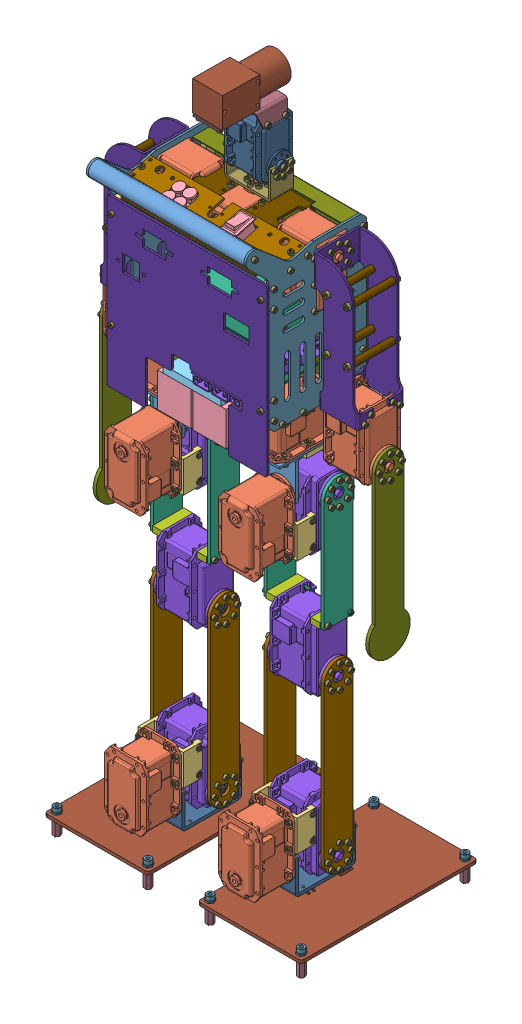
SolidWorks assembly 机器人, configuration 默认. Lengths in mm. (continued)
Components (placement in the parent): (continued)
- 左腿-1: 左腿 [默认] at (1223.8429 -132.4302 49.3314) x (0.483512 -0.009844 -0.875282) z (0.842178 0.277849 0.4621) size (197.18 402.23 253.32) (continued)
  - hexagon socket head cap screws gb-41: hexagon socket head cap screws gb [GB_FASTENER_SCREWS_HSHCS M2.5X6-N] at (-141.6338 221.8483 -139.9557) x (-0.009844 0.960574 0.277849) z (-0.277849 -0.269548 0.922033) size (8.5 4.5 4.5)
  - hexagon socket head cap screws gb-42: hexagon socket head cap screws gb [GB_FASTENER_SCREWS_HSHCS M2.5X6-N] at (-152.2711 227.0985 -158.4836) x (-0.009844 0.960574 0.277849) z (-0.277849 -0.269548 0.922033) size (8.5 4.5 4.5)
  - hexagon socket head cap screws gb-43: hexagon socket head cap screws gb [GB_FASTENER_SCREWS_HSHCS M2.5X6-N] at (-124.262 231.6628 -173.2708) x (-0.009844 0.960574 0.277849) z (-0.277849 -0.269548 0.922033) size (8.5 4.5 4.5)
  - hexagon socket head cap screws gb-44: hexagon socket head cap screws gb [GB_FASTENER_SCREWS_HSHCS M2.5X6-N] at (-113.6248 226.4125 -154.7429) x (-0.009844 0.960574 0.277849) z (-0.277849 -0.269548 0.922033) size (8.5 4.5 4.5)
  - hexagon socket head cap screws gb-45: hexagon socket head cap screws gb [GB_FASTENER_SCREWS_HSHCS M2.5X6-N] at (-151.57 247.2943 -140.1019) x (-0.875282 -0.142634 0.4621) z (-0.4621 0.528483 -0.712158) size (8.5 4.5 4.5)
  - hexagon socket head cap screws gb-46: hexagon socket head cap screws gb [GB_FASTENER_SCREWS_HSHCS M2.5X6-N] at (-147.8409 248.5328 -132.6561) x (-0.875282 -0.142634 0.4621) z (-0.4621 0.528483 -0.712158) size (8.5 4.5 4.5)
  - hexagon socket head cap screws gb-47: hexagon socket head cap screws gb [GB_FASTENER_SCREWS_HSHCS M2.5X6-N] at (-146.3597 255.2355 -127.7816) x (-0.875282 -0.142634 0.4621) z (-0.4621 0.528483 -0.712158) size (8.5 4.5 4.5)
  - hexagon socket head cap screws gb-50: hexagon socket head cap screws gb [GB_FASTENER_SCREWS_HSHCS M2.5X6-N] at (-150.9798 554.3402 -44.2096) x (-0.875282 -0.142634 0.4621) z (-0.4621 0.528483 -0.712158) size (8.5 4.5 4.5)
  - hexagon socket head cap screws gb-51: hexagon socket head cap screws gb [GB_FASTENER_SCREWS_HSHCS M2.5X6-N] at (-154.7723 559.2912 -49.865) x (-0.875282 -0.142634 0.4621) z (-0.4621 0.528483 -0.712158) size (8.5 4.5 4.5)
  - hexagon socket head cap screws gb-52: hexagon socket head cap screws gb [GB_FASTENER_SCREWS_HSHCS M2.5X6-N] at (-149.3454 546.0998 -43.6574) x (-0.875282 -0.142634 0.4621) z (-0.4621 0.528483 -0.712158) size (8.5 4.5 4.5)
  - hexagon socket head cap screws gb-54: hexagon socket head cap screws gb [GB_FASTENER_SCREWS_HSHCS M2.5X6-N] at (-141.4858 262.0369 -179.1169) x (0.483512 -0.238647 0.842178) z (-0.842178 0.135478 0.521902) size (8.5 4.5 4.5)
  - hexagon socket head cap screws gb-55: hexagon socket head cap screws gb [GB_FASTENER_SCREWS_HSHCS M2.5X6-N] at (-138.7424 269.9679 -178.4445) x (0.483512 -0.238647 0.842178) z (-0.842178 0.135478 0.521902) size (8.5 4.5 4.5)
  - hexagon socket head cap screws gb-56: hexagon socket head cap screws gb [GB_FASTENER_SCREWS_HSHCS M2.5X6-N] at (-141.6389 276.9799 -174.7946) x (0.483512 -0.238647 0.842178) z (-0.842178 0.135478 0.521902) size (8.5 4.5 4.5)
  - hexagon socket head cap screws gb-57: hexagon socket head cap screws gb [GB_FASTENER_SCREWS_HSHCS M2.5X6-N] at (-148.4787 278.9653 -170.3051) x (0.483512 -0.238647 0.842178) z (-0.842178 0.135478 0.521902) size (8.5 4.5 4.5)
  - hexagon socket head cap screws gb-58: hexagon socket head cap screws gb [GB_FASTENER_SCREWS_HSHCS M2.5X6-N] at (-148.2622 257.8326 -176.4177) x (0.483512 -0.238647 0.842178) z (-0.842178 0.135478 0.521902) size (8.5 4.5 4.5)
  - hexagon socket head cap screws gb-59: hexagon socket head cap screws gb [GB_FASTENER_SCREWS_HSHCS M2.5X6-N] at (-155.102 259.818 -171.9283) x (0.483512 -0.238647 0.842178) z (-0.842178 0.135478 0.521902) size (8.5 4.5 4.5)
  - hexagon socket head cap screws gb-60: hexagon socket head cap screws gb [GB_FASTENER_SCREWS_HSHCS M2.5X6-N] at (-157.9986 266.83 -168.2783) x (0.483512 -0.238647 0.842178) z (-0.842178 0.135478 0.521902) size (8.5 4.5 4.5)
  - hexagon socket head cap screws gb-61: hexagon socket head cap screws gb [GB_FASTENER_SCREWS_HSHCS M2.5X6-N] at (-155.2551 274.761 -167.606) x (0.483512 -0.238647 0.842178) z (-0.842178 0.135478 0.521902) size (8.5 4.5 4.5)
  - hexagon socket head cap screws gb-62: hexagon socket head cap screws gb [GB_FASTENER_SCREWS_HSHCS M2.5X6-N] at (-140.219 414.0541 -136.7672) x (0.483512 -0.238647 0.842178) z (-0.842178 0.135478 0.521902) size (8.5 4.5 4.5)
  - hexagon socket head cap screws gb-63: hexagon socket head cap screws gb [GB_FASTENER_SCREWS_HSHCS M2.5X6-N] at (-142.9624 406.123 -137.4396) x (0.483512 -0.238647 0.842178) z (-0.842178 0.135478 0.521902) size (8.5 4.5 4.5)
  - hexagon socket head cap screws gb-64: hexagon socket head cap screws gb [GB_FASTENER_SCREWS_HSHCS M2.5X6-N] at (-149.7388 401.9188 -134.7405) x (0.483512 -0.238647 0.842178) z (-0.842178 0.135478 0.521902) size (8.5 4.5 4.5)
  - hexagon socket head cap screws gb-65: hexagon socket head cap screws gb [GB_FASTENER_SCREWS_HSHCS M2.5X6-N] at (-156.5786 403.9042 -130.251) x (0.483512 -0.238647 0.842178) z (-0.842178 0.135478 0.521902) size (8.5 4.5 4.5)
  - hexagon socket head cap screws gb-66: hexagon socket head cap screws gb [GB_FASTENER_SCREWS_HSHCS M2.5X6-N] at (-159.4752 410.9161 -126.601) x (0.483512 -0.238647 0.842178) z (-0.842178 0.135478 0.521902) size (8.5 4.5 4.5)
  - hexagon socket head cap screws gb-67: hexagon socket head cap screws gb [GB_FASTENER_SCREWS_HSHCS M2.5X6-N] at (-156.7318 418.8472 -125.9287) x (0.483512 -0.238647 0.842178) z (-0.842178 0.135478 0.521902) size (8.5 4.5 4.5)
  - hexagon socket head cap screws gb-68: hexagon socket head cap screws gb [GB_FASTENER_SCREWS_HSHCS M2.5X6-N] at (-149.9554 423.0514 -128.6278) x (0.483512 -0.238647 0.842178) z (-0.842178 0.135478 0.521902) size (8.5 4.5 4.5)
  - hexagon socket head cap screws gb-69: hexagon socket head cap screws gb [GB_FASTENER_SCREWS_HSHCS M2.5X6-N] at (-143.1156 421.0661 -133.1173) x (0.483512 -0.238647 0.842178) z (-0.842178 0.135478 0.521902) size (8.5 4.5 4.5)
  - hexagon socket head cap screws gb-70: hexagon socket head cap screws gb [GB_FASTENER_SCREWS_HSHCS M2.5X6-N] at (-141.7281 560.8323 -94.3204) x (0.483512 -0.238647 0.842178) z (-0.842178 0.135478 0.521902) size (8.5 4.5 4.5)
  - hexagon socket head cap screws gb-71: hexagon socket head cap screws gb [GB_FASTENER_SCREWS_HSHCS M2.5X6-N] at (-144.4715 552.9012 -94.9927) x (0.483512 -0.238647 0.842178) z (-0.842178 0.135478 0.521902) size (8.5 4.5 4.5)
  - hexagon socket head cap screws gb-72: hexagon socket head cap screws gb [GB_FASTENER_SCREWS_HSHCS M2.5X6-N] at (-151.2479 548.697 -92.2936) x (0.483512 -0.238647 0.842178) z (-0.842178 0.135478 0.521902) size (8.5 4.5 4.5)
  - hexagon socket head cap screws gb-73: hexagon socket head cap screws gb [GB_FASTENER_SCREWS_HSHCS M2.5X6-N] at (-158.0877 550.6823 -87.8041) x (0.483512 -0.238647 0.842178) z (-0.842178 0.135478 0.521902) size (8.5 4.5 4.5)
  - hexagon socket head cap screws gb-74: hexagon socket head cap screws gb [GB_FASTENER_SCREWS_HSHCS M2.5X6-N] at (-160.9843 557.6943 -84.1542) x (0.483512 -0.238647 0.842178) z (-0.842178 0.135478 0.521902) size (8.5 4.5 4.5)
  - hexagon socket head cap screws gb-75: hexagon socket head cap screws gb [GB_FASTENER_SCREWS_HSHCS M2.5X6-N] at (-158.2408 565.6254 -83.4818) x (0.483512 -0.238647 0.842178) z (-0.842178 0.135478 0.521902) size (8.5 4.5 4.5)
  - hexagon socket head cap screws gb-76: hexagon socket head cap screws gb [GB_FASTENER_SCREWS_HSHCS M2.5X6-N] at (-151.4645 569.8296 -86.1809) x (0.483512 -0.238647 0.842178) z (-0.842178 0.135478 0.521902) size (8.5 4.5 4.5)
  - hexagon socket head cap screws gb-77: hexagon socket head cap screws gb [GB_FASTENER_SCREWS_HSHCS M2.5X6-N] at (-144.6246 567.8442 -90.6704) x (0.483512 -0.238647 0.842178) z (-0.842178 0.135478 0.521902) size (8.5 4.5 4.5)
  - hexagon socket head cap screws gb-80: hexagon socket head cap screws gb [GB_FASTENER_SCREWS_HSHCS M2.5X6-N] at (-158.5014 558.0527 -57.3108) x (-0.875282 -0.142634 0.4621) z (-0.4621 0.528483 -0.712158) size (8.5 4.5 4.5)
  - hexagon socket head cap screws gb-81: hexagon socket head cap screws gb [GB_FASTENER_SCREWS_HSHCS M2.5X6-N] at (-159.9827 551.35 -62.1853) x (-0.875282 -0.142634 0.4621) z (-0.4621 0.528483 -0.712158) size (8.5 4.5 4.5)
  - hexagon socket head cap screws gb-82: hexagon socket head cap screws gb [GB_FASTENER_SCREWS_HSHCS M2.5X6-N] at (-155.3626 252.2453 -145.7573) x (-0.875282 -0.142634 0.4621) z (-0.4621 0.528483 -0.712158) size (8.5 4.5 4.5)
  - hexagon socket head cap screws gb-83: hexagon socket head cap screws gb [GB_FASTENER_SCREWS_HSHCS M2.5X6-N] at (-156.9969 260.4857 -146.3095) x (-0.875282 -0.142634 0.4621) z (-0.4621 0.528483 -0.712158) size (8.5 4.5 4.5)
  - hexagon socket head cap screws gb-85: hexagon socket head cap screws gb [GB_FASTENER_SCREWS_HSHCS M2.5X6-N] at (-131.9016 563.4253 -88.5406) x (0.483512 -0.238647 0.842178) z (-0.842178 0.135478 0.521902) size (8.5 4.5 4.5)
  - hexagon socket head cap screws gb-86: hexagon socket head cap screws gb [GB_FASTENER_SCREWS_HSHCS M2.5X6-N] at (-131.685 542.2927 -94.6533) x (0.483512 -0.238647 0.842178) z (-0.842178 0.135478 0.521902) size (8.5 4.5 4.5)
  - hexagon socket head cap screws gb-87: hexagon socket head cap screws gb [GB_FASTENER_SCREWS_HSHCS M2.5X6-N] at (-110.1435 552.6862 -50.6426) x (-0.483512 0.238647 -0.842178) z (0.842178 0.389134 -0.373244) size (8.5 4.5 4.5)
  - hexagon socket head cap screws gb-88: hexagon socket head cap screws gb [GB_FASTENER_SCREWS_HSHCS M2.5X6-N] at (-109.9269 531.5536 -56.7553) x (-0.483512 0.238647 -0.842178) z (0.842178 0.389134 -0.373244) size (8.5 4.5 4.5)
  - hexagon socket head cap screws gb-89: hexagon socket head cap screws gb [GB_FASTENER_SCREWS_HSHCS M2.5X6-N] at (-140.3084 526.6662 -40.935) x (-0.483512 0.238647 -0.842178) z (0.842178 0.389134 -0.373244) size (8.5 4.5 4.5)
  - hexagon socket head cap screws gb-90: hexagon socket head cap screws gb [GB_FASTENER_SCREWS_HSHCS M2.5X6-N] at (-140.0918 505.5335 -47.0477) x (-0.483512 0.238647 -0.842178) z (0.842178 0.389134 -0.373244) size (8.5 4.5 4.5)
  - hexagon socket head cap screws gb-91: hexagon socket head cap screws gb [GB_FASTENER_SCREWS_HSHCS M2.5X6-N] at (-161.6565 516.1772 -84.6088) x (0.483512 -0.238647 0.842178) z (-0.842178 0.135478 0.521902) size (8.5 4.5 4.5)
  - hexagon socket head cap screws gb-92: hexagon socket head cap screws gb [GB_FASTENER_SCREWS_HSHCS M2.5X6-N] at (-161.873 537.3098 -78.4962) x (0.483512 -0.238647 0.842178) z (-0.842178 0.135478 0.521902) size (8.5 4.5 4.5)
  - hexagon socket head cap screws gb-93: hexagon socket head cap screws gb [GB_FASTENER_SCREWS_HSHCS M2.5X6-N] at (-129.0537 286.009 -168.7749) x (0.483512 -0.238647 0.842178) z (-0.842178 0.135478 0.521902) size (8.5 4.5 4.5)
  - hexagon socket head cap screws gb-94: hexagon socket head cap screws gb [GB_FASTENER_SCREWS_HSHCS M2.5X6-N] at (-128.8371 264.8764 -174.8875) x (0.483512 -0.238647 0.842178) z (-0.842178 0.135478 0.521902) size (8.5 4.5 4.5)
  - hexagon socket head cap screws gb-95: hexagon socket head cap screws gb [GB_FASTENER_SCREWS_HSHCS M2.5X6-N] at (-159.4583 302.1588 -146.5051) x (0.483512 -0.238647 0.842178) z (-0.842178 0.135478 0.521902) size (8.5 4.5 4.5)
  - hexagon socket head cap screws gb-96: hexagon socket head cap screws gb [GB_FASTENER_SCREWS_HSHCS M2.5X6-N] at (-159.2417 281.0262 -152.6178) x (0.483512 -0.238647 0.842178) z (-0.842178 0.135478 0.521902) size (8.5 4.5 4.5)
  - hexagon socket head cap screws gb-97: hexagon socket head cap screws gb [GB_FASTENER_SCREWS_HSHCS M2.5X6-N] at (-107.2956 275.2699 -130.8769) x (-0.483512 0.238647 -0.842178) z (0.842178 0.389134 -0.373244) size (8.5 4.5 4.5)
  - hexagon socket head cap screws gb-98: hexagon socket head cap screws gb [GB_FASTENER_SCREWS_HSHCS M2.5X6-N] at (-107.079 254.1373 -136.9895) x (-0.483512 0.238647 -0.842178) z (0.842178 0.389134 -0.373244) size (8.5 4.5 4.5)
  - hexagon socket head cap screws gb-99: hexagon socket head cap screws gb [GB_FASTENER_SCREWS_HSHCS M2.5X6-N] at (-137.6771 270.3825 -115.0566) x (-0.483512 0.238647 -0.842178) z (0.842178 0.389134 -0.373244) size (8.5 4.5 4.5)
  - hexagon socket head cap screws gb-100: hexagon socket head cap screws gb [GB_FASTENER_SCREWS_HSHCS M2.5X6-N] at (-137.8937 291.5152 -108.944) x (-0.483512 0.238647 -0.842178) z (0.842178 0.389134 -0.373244) size (8.5 4.5 4.5)
  - hexagon socket head cap screws gb-101: hexagon socket head cap screws gb [GB_FASTENER_SCREWS_HSHCS M2.5X6-N] at (-158.4296 289.7559 -103.5894) x (0.875282 0.142634 -0.4621) z (0.4621 0.035147 0.886131) size (8.5 4.5 4.5)
  - hexagon socket head cap screws gb-102: hexagon socket head cap screws gb [GB_FASTENER_SCREWS_HSHCS M2.5X6-N] at (-158.213 268.6232 -109.7021) x (0.875282 0.142634 -0.4621) z (0.4621 0.035147 0.886131) size (8.5 4.5 4.5)
  - hexagon socket head cap screws gb-103: hexagon socket head cap screws gb [GB_FASTENER_SCREWS_HSHCS M2.5X6-N] at (-175.1591 298.0131 -132.7287) x (0.875282 0.142634 -0.4621) z (0.4621 0.035147 0.886131) size (8.5 4.5 4.5)
  - hexagon socket head cap screws gb-104: hexagon socket head cap screws gb [GB_FASTENER_SCREWS_HSHCS M2.5X6-N] at (-174.9425 276.8804 -138.8414) x (0.875282 0.142634 -0.4621) z (0.4621 0.035147 0.886131) size (8.5 4.5 4.5)
  - hexagon socket head cap screws gb-105: hexagon socket head cap screws gb [GB_FASTENER_SCREWS_HSHCS M2.5X6-N] at (-177.7314 533.1384 -64.6366) x (0.875282 0.142634 -0.4621) z (0.4621 0.035147 0.886131) size (8.5 4.5 4.5)
  - hexagon socket head cap screws gb-106: hexagon socket head cap screws gb [GB_FASTENER_SCREWS_HSHCS M2.5X6-N] at (-177.5148 512.0058 -70.7493) x (0.875282 0.142634 -0.4621) z (0.4621 0.035147 0.886131) size (8.5 4.5 4.5)
  - hexagon socket head cap screws gb-107: hexagon socket head cap screws gb [GB_FASTENER_SCREWS_HSHCS M2.5X6-N] at (-161.0019 524.8812 -35.4973) x (0.875282 0.142634 -0.4621) z (0.4621 0.035147 0.886131) size (8.5 4.5 4.5)
  - hexagon socket head cap screws gb-108: hexagon socket head cap screws gb [GB_FASTENER_SCREWS_HSHCS M2.5X6-N] at (-160.7853 503.7486 -41.6099) x (0.875282 0.142634 -0.4621) z (0.4621 0.035147 0.886131) size (8.5 4.5 4.5)
  - hexagon socket head cap screws gb-112: hexagon socket head cap screws gb [GB_FASTENER_SCREWS_HSHCS M2.5X6-N] at (-110.2235 444.9324 -70.4204) x (-0.483512 0.238647 -0.842178) z (0.842178 0.389134 -0.373244) size (8.5 4.5 4.5)
  - hexagon socket head cap screws gb-113: hexagon socket head cap screws gb [GB_FASTENER_SCREWS_HSHCS M2.5X6-N] at (-129.4797 441.7945 -60.2542) x (-0.483512 0.238647 -0.842178) z (0.842178 0.389134 -0.373244) size (8.5 4.5 4.5)
  - hexagon socket head cap screws gb-114: hexagon socket head cap screws gb [GB_FASTENER_SCREWS_HSHCS M2.5X6-N] at (-140.6944 459.9719 -123.4945) x (0.483512 -0.238647 0.842178) z (-0.842178 0.135478 0.521902) size (8.5 4.5 4.5)
  - hexagon socket head cap screws gb-115: hexagon socket head cap screws gb [GB_FASTENER_SCREWS_HSHCS M2.5X6-N] at (-159.9506 456.834 -113.3283) x (0.483512 -0.238647 0.842178) z (-0.842178 0.135478 0.521902) size (8.5 4.5 4.5)
  - hexagon socket head cap screws gb-116: hexagon socket head cap screws gb [GB_FASTENER_SCREWS_HSHCS M2.5X6-N] at (-109.7795 556.0392 -76.6179) x (-0.875282 -0.142634 0.4621) z (-0.4621 0.528483 -0.712158) size (8.5 4.5 4.5)
  - hexagon socket head cap screws gb-117: hexagon socket head cap screws gb [GB_FASTENER_SCREWS_HSHCS M2.5X6-N] at (-122.5485 545.0447 -39.0603) x (-0.483512 0.238647 -0.842178) z (0.842178 0.389134 -0.373244) size (8.5 4.5 4.5)
  - hexagon socket head cap screws gb-118: hexagon socket head cap screws gb [GB_FASTENER_SCREWS_HSHCS M2.5X6-N] at (-121.0395 398.2665 -81.5072) x (-0.483512 0.238647 -0.842178) z (0.842178 0.389134 -0.373244) size (8.5 4.5 4.5)
  - hexagon socket head cap screws gb-119: hexagon socket head cap screws gb [GB_FASTENER_SCREWS_HSHCS M2.5X6-N] at (-119.5628 254.1804 -123.1844) x (-0.483512 0.238647 -0.842178) z (0.842178 0.389134 -0.373244) size (8.5 4.5 4.5)
  - hexagon socket head cap screws gb-120: hexagon socket head cap screws gb [GB_FASTENER_SCREWS_HSHCS M2.5X6-N] at (-106.7938 265.1749 -160.742) x (-0.875282 -0.142634 0.4621) z (-0.4621 0.528483 -0.712158) size (8.5 4.5 4.5)
  - 脚钉铜柱-1: 脚钉铜柱 [默认] at (-43.7122 221.3339 -179.6967) x (0.999951 0.009844 0.001395) z (0.001395 -0.277849 0.960624) size (6.82 21 6.51)
  - 脚钉铜柱-2: 脚钉铜柱 [默认] at (-182.0068 198.7978 -106.6849) x (0.999951 0.009844 0.001395) z (0.001395 -0.277849 0.960624) size (6.82 21 6.51)
  - 脚钉铜柱-3: 脚钉铜柱 [默认] at (-224.5559 219.7987 -180.7966) x (0.999951 0.009844 0.001395) z (0.001395 -0.277849 0.960624) size (6.82 21 6.51)
  - 脚钉铜柱-4: 脚钉铜柱 [默认] at (-86.2613 242.3349 -253.8084) x (0.999951 0.009844 0.001395) z (0.001395 -0.277849 0.960624) size (6.82 21 6.51)
  - prevailing torque type style 1 gb-1: prevailing torque type style 1 gb [GB_HEXAGON_TYPE9 M4-N] at (-182.2069 218.3167 -101.039) x (0.999924 0.0074 0.009844) z (-0.009844 0.960574 0.277849) size (8.08 7 6)
  - prevailing torque type style 1 gb-2: prevailing torque type style 1 gb [GB_HEXAGON_TYPE9 M4-N] at (-43.9122 240.8528 -174.0508) x (0.999924 0.0074 0.009844) z (-0.009844 0.960574 0.277849) size (8.08 7 6)
  - prevailing torque type style 1 gb-3: prevailing torque type style 1 gb [GB_HEXAGON_TYPE9 M4-N] at (-224.7559 239.3176 -175.1507) x (0.999924 0.0074 0.009844) z (-0.009844 0.960574 0.277849) size (8.08 7 6)
  - prevailing torque type style 1 gb-4: prevailing torque type style 1 gb [GB_HEXAGON_TYPE9 M4-N] at (-86.4613 261.8537 -248.1625) x (0.999924 0.0074 0.009844) z (-0.009844 0.960574 0.277849) size (8.08 7 6)
- 手臂-1: 手臂 [默认] at (884.6916 966.1212 206.2056) x (-0.996132 -0.087558 0.007426) z (-0.009574 0.192154 0.981318) size (79.62 325.5 103.6)
  - 机器人-下臂骨-1: 机器人-下臂骨 [默认] at (47.1501 636.0849 -272.5502) x (-0.087558 -0.977451 0.192154) z (-0.007426 -0.192249 -0.981318) size (174 3 40)
  - 机器人-上臂骨-1: 机器人-上臂骨 [默认] at (-27.1879 355.8538 -217.4953) x (0.996132 -0.087349 0.009574) z (-0.007426 -0.192249 -0.981318) size (43.55 128 44.76)
  - MX64-1: MX64 [默认] at (8.4945 501.5565 -245.9023) x (-0.007426 -0.192249 -0.981318) z (0.996132 -0.087349 0.009574) size (40.2 62.1 50)
  - hexagon socket head cap screws gb-9: hexagon socket head cap screws gb [GB_FASTENER_SCREWS_HSHCS M2.5X6-N] at (36.4192 488.2714 -243.5109) x (-0.996132 0.087349 -0.009574) z (0.009574 0.21619 0.976304) size (8.5 4.5 4.5)
  - hexagon socket head cap screws gb-10: hexagon socket head cap screws gb [GB_FASTENER_SCREWS_HSHCS M2.5X6-N] at (36.6435 489.9252 -251.7629) x (-0.996132 0.087349 -0.009574) z (0.009574 0.21619 0.976304) size (8.5 4.5 4.5)
  - hexagon socket head cap screws gb-11: hexagon socket head cap screws gb [GB_FASTENER_SCREWS_HSHCS M2.5X6-N] at (37.3006 496.9086 -256.4191) x (-0.996132 0.087349 -0.009574) z (0.009574 0.21619 0.976304) size (8.5 4.5 4.5)
  - hexagon socket head cap screws gb-12: hexagon socket head cap screws gb [GB_FASTENER_SCREWS_HSHCS M2.5X6-N] at (38.0056 505.1308 -254.7521) x (-0.996132 0.087349 -0.009574) z (0.009574 0.21619 0.976304) size (8.5 4.5 4.5)
  - hexagon socket head cap screws gb-13: hexagon socket head cap screws gb [GB_FASTENER_SCREWS_HSHCS M2.5X6-N] at (38.3455 509.7753 -247.7383) x (-0.996132 0.087349 -0.009574) z (0.009574 0.21619 0.976304) size (8.5 4.5 4.5)
  - hexagon socket head cap screws gb-14: hexagon socket head cap screws gb [GB_FASTENER_SCREWS_HSHCS M2.5X6-N] at (38.1211 508.1215 -239.4864) x (-0.996132 0.087349 -0.009574) z (0.009574 0.21619 0.976304) size (8.5 4.5 4.5)
  - hexagon socket head cap screws gb-15: hexagon socket head cap screws gb [GB_FASTENER_SCREWS_HSHCS M2.5X6-N] at (37.464 501.1381 -234.8301) x (-0.996132 0.087349 -0.009574) z (0.009574 0.21619 0.976304) size (8.5 4.5 4.5)
  - hexagon socket head cap screws gb-16: hexagon socket head cap screws gb [GB_FASTENER_SCREWS_HSHCS M2.5X6-N] at (36.759 492.9159 -236.4971) x (-0.996132 0.087349 -0.009574) z (0.009574 0.21619 0.976304) size (8.5 4.5 4.5)
  - 垫柱-1: 垫柱 [默认] at (-13.783 364.6841 -239.3277) x (0.999972 -0.000721 -0.007426) z (0.007426 0.192249 0.981318) size (6 6 40)
  - 垫柱-2: 垫柱 [默认] at (6.1396 362.9371 -239.1362) x (0.999972 -0.000721 -0.007426) z (0.007426 0.192249 0.981318) size (6 6 40)
  - 垫柱-3: 垫柱 [默认] at (-9.4051 413.5566 -248.9354) x (0.999972 -0.000721 -0.007426) z (0.007426 0.192249 0.981318) size (6 6 40)
  - 垫柱-4: 垫柱 [默认] at (10.5175 411.8096 -248.7439) x (0.999972 -0.000721 -0.007426) z (0.007426 0.192249 0.981318) size (6 6 40)
- 手臂-2: 手臂 [默认] at (1172.1888 966.1212 -84.237) x (0.996132 -0.087558 -0.007426) z (0.009574 0.192154 -0.981318) size (79.62 325.5 103.6)
  - 机器人-下臂骨-1: 机器人-下臂骨 [默认] at (47.1501 636.0849 -272.5502) x (-0.087558 -0.977451 0.192154) z (-0.007426 -0.192249 -0.981318) size (174 3 40)
  - 机器人-上臂骨-1: 机器人-上臂骨 [默认] at (-27.1879 355.8538 -217.4953) x (0.996132 -0.087349 0.009574) z (-0.007426 -0.192249 -0.981318) size (43.55 128 44.76)
  - MX64-1: MX64 [默认] at (8.4945 501.5565 -245.9023) x (-0.007426 -0.192249 -0.981318) z (0.996132 -0.087349 0.009574) size (40.2 62.1 50)
  - hexagon socket head cap screws gb-9: hexagon socket head cap screws gb [GB_FASTENER_SCREWS_HSHCS M2.5X6-N] at (36.4192 488.2714 -243.5109) x (-0.996132 0.087349 -0.009574) z (0.009574 0.21619 0.976304) size (8.5 4.5 4.5)
  - hexagon socket head cap screws gb-10: hexagon socket head cap screws gb [GB_FASTENER_SCREWS_HSHCS M2.5X6-N] at (36.6435 489.9252 -251.7629) x (-0.996132 0.087349 -0.009574) z (0.009574 0.21619 0.976304) size (8.5 4.5 4.5)
  - hexagon socket head cap screws gb-11: hexagon socket head cap screws gb [GB_FASTENER_SCREWS_HSHCS M2.5X6-N] at (37.3006 496.9086 -256.4191) x (-0.996132 0.087349 -0.009574) z (0.009574 0.21619 0.976304) size (8.5 4.5 4.5)
  - hexagon socket head cap screws gb-12: hexagon socket head cap screws gb [GB_FASTENER_SCREWS_HSHCS M2.5X6-N] at (38.0056 505.1308 -254.7521) x (-0.996132 0.087349 -0.009574) z (0.009574 0.21619 0.976304) size (8.5 4.5 4.5)
  - hexagon socket head cap screws gb-13: hexagon socket head cap screws gb [GB_FASTENER_SCREWS_HSHCS M2.5X6-N] at (38.3455 509.7753 -247.7383) x (-0.996132 0.087349 -0.009574) z (0.009574 0.21619 0.976304) size (8.5 4.5 4.5)
  - hexagon socket head cap screws gb-14: hexagon socket head cap screws gb [GB_FASTENER_SCREWS_HSHCS M2.5X6-N] at (38.1211 508.1215 -239.4864) x (-0.996132 0.087349 -0.009574) z (0.009574 0.21619 0.976304) size (8.5 4.5 4.5)
  - hexagon socket head cap screws gb-15: hexagon socket head cap screws gb [GB_FASTENER_SCREWS_HSHCS M2.5X6-N] at (37.464 501.1381 -234.8301) x (-0.996132 0.087349 -0.009574) z (0.009574 0.21619 0.976304) size (8.5 4.5 4.5)
  - hexagon socket head cap screws gb-16: hexagon socket head cap screws gb [GB_FASTENER_SCREWS_HSHCS M2.5X6-N] at (36.759 492.9159 -236.4971) x (-0.996132 0.087349 -0.009574) z (0.009574 0.21619 0.976304) size (8.5 4.5 4.5)
  - 垫柱-1: 垫柱 [默认] at (-13.783 364.6841 -239.3277) x (0.999972 -0.000721 -0.007426) z (0.007426 0.192249 0.981318) size (6 6 40)
  - 垫柱-2: 垫柱 [默认] at (6.1396 362.9371 -239.1362) x (0.999972 -0.000721 -0.007426) z (0.007426 0.192249 0.981318) size (6 6 40)
  - 垫柱-3: 垫柱 [默认] at (-9.4051 413.5566 -248.9354) x (0.999972 -0.000721 -0.007426) z (0.007426 0.192249 0.981318) size (6 6 40)
  - 垫柱-4: 垫柱 [默认] at (10.5175 411.8096 -248.7439) x (0.999972 -0.000721 -0.007426) z (0.007426 0.192249 0.981318) size (6 6 40)
- 躯干-1: 躯干 [默认] at (1014.3063 415.9938 -67.5657) size (172 287.24 163.85)
  - 机器人-下腰骨-1: 机器人-下腰骨 [默认] at (14.1339 4.9855 143.3) size (150 2 94.2)
  - 机器人-腰部连接件-1: 机器人-腰部连接件 [默认] at (86.3339 40.9855 146.55) size (5.6 6 68)
  - 机器人-腰部连接件-2: 机器人-腰部连接件 [默认] at (-58.0661 40.9855 146.55) size (5.6 6 68)
  - 机器人-腰部支撑件-1: 机器人-腰部支撑件 [默认] at (69.0339 0.6855 128.55) x (0 0 -1) z (1 0 0) size (40 4.3 40.2)
  - 机器人-腰部支撑件-2: 机器人-腰部支撑件 [默认] at (-40.7661 0.6855 128.55) x (0 0 -1) z (1 0 0) size (40 4.3 40.2)
  - 电池组-1: 电池组 [默认] at (-73.6661 8.3922 158.5613) x (0 -1 0) z (1 0 0) size (40 92 66)
    - 大电池-1: 大电池 [默认] at (-15.0933 -28.8887 72) size (33 78 32)
    - 大电池-2: 大电池 [默认] at (-15.0933 -28.8887 106) size (33 78 32)
    - 小电池-1: 小电池 [默认] at (-35.0933 63.1113 89) x (0 0 1) z (0 -1 0) size (56 7 92)
  - 电路-1: 电路 [默认] at (-149.9254 121.6563 46.2423) x (0.629094 0.186421 -0.754644) z (0.775792 -0.211602 0.594451) size (135.66 81.1 136.29)
    - TX2-1: TX2 [默认] at (66.6739 -13.371 209.1651) x (-0.629094 -0.048866 -0.775792) z (0.186421 0.959412 -0.211602) size (87.07 50.04 32.13)
    - 9003-1: 9003 [默认] at (15.6894 -27.7493 144.427) x (0.629094 0.048866 0.775792) z (-0.186421 -0.959412 0.211602) size (96.22 72.67 50.58)
    - Main-1: Main [默认] at (20.5563 -29.3993 193.2183) x (0.629094 0.048866 0.775792) z (0.186421 0.959412 -0.211602) size (100 91.07 21.61)
  - 机器人-背板-1: 机器人-背板 [默认] at (14.1339 173.2258 167.0875) x (1 0 0) z (0 -0.258819 0.965926) size (150 2 40)
  - 脑袋-1: 脑袋 [默认] at (31.3694 207.3211 170.3695) x (-0.999965 0 -0.008321) z (0.008321 0 -0.999965) size (45.6 104.22 67.8)
    - MX28-2-1: MX28-2 [默认] at (67.0789 12.1977 37.204) x (0 0 -1) z (-1 0 0) size (35.6 50.71 44.45)
    - 工业摄像头-1: 工业摄像头 [默认] at (17.9784 61.4039 35.5741) x (-1 0 0) z (0 1 0) size (29 65.7 29)
    - 机器人-脖子-1: 机器人-脖子 [默认] at (17.6701 -26.3128 48.8741) size (44.75 27.37 22)
    - 机器人-摄像头固定件-1: 机器人-摄像头固定件 [默认] at (17.9784 46.9039 59.8741) x (-1 0 0) z (0 1 0) size (33.15 61 17.05)
  - 机器人-侧板-3: 机器人-侧板 [默认] at (-60.8661 139.1722 141.05) x (0 0 1) z (-1 0 0) size (116.15 161.21 2)
  - 机器人-侧板-4: 机器人-侧板 [默认] at (91.1339 139.1722 141.05) x (0 0 1) z (-1 0 0) size (116.15 161.21 2)
  - 机器人-上腰骨-2: 机器人-上腰骨 [默认] at (14.1339 48.9855 149.05) size (100.8 2 61)
  - 机器人-前盖-2: 机器人-前盖 [默认] at (14.1339 110.9855 94.95) x (1 0 0) z (0 -1 0) size (154 19.53 171.5)
  - 机器人-后盖-2: 机器人-后盖 [默认] at (14.1339 100.9855 188.95) size (154 160 2)
  - 机器人-肩骨-1: 机器人-肩骨 [默认] at (-24.8661 182.5355 128.55) size (28.68 11.38 40.2)
  - 机器人-肩骨-2: 机器人-肩骨 [默认] at (53.1339 182.5355 128.55) x (-1 0 0) z (0 0 -1) size (28.68 11.38 40.2)
  - 提手-1: 提手 [默认] at (-60.8661 194.6934 203.5985) size (150 15 15)
  - MX64-1: MX64 [默认] at (69.0339 23.9855 128.55) x (-1 0 0) z (0 -1 0) size (40.2 62.1 50)
  - MX64-2: MX64 [默认] at (-40.7661 23.9855 128.55) x (-1 0 0) z (0 -1 0) size (40.2 62.1 50)
  - MX28-3: MX28 [默认] at (22.2109 109.2267 134.6509) x (1 0 0) z (0 1 0) size (35.6 50.71 42.85)
  - MX64-3: MX64 [默认] at (-43.8661 162.8855 128.55) x (0 0 1) z (-1 0 0) size (40.2 62.1 50)
  - MX64-4: MX64 [默认] at (72.1339 162.8855 128.55) x (0 0 -1) z (1 0 0) size (40.2 62.1 50)
  - 机器人-盖子连接件-1: 机器人-盖子连接件 [默认] at (86.1339 152.4855 184.95) size (6 22 8)
  - 机器人-盖子连接件-2: 机器人-盖子连接件 [默认] at (86.1339 59.4855 184.95) size (6 22 8)
  - 机器人-盖子连接件-3: 机器人-盖子连接件 [默认] at (-57.8661 59.4855 184.95) size (6 22 8)
  - 机器人-盖子连接件-4: 机器人-盖子连接件 [默认] at (-57.8661 152.4855 184.95) size (6 22 8)
  - 机器人-盖子连接件-5: 机器人-盖子连接件 [默认] at (86.1339 162.4855 98.95) size (6 22 8)
  - 机器人-盖子连接件-6: 机器人-盖子连接件 [默认] at (86.1339 59.4855 98.95) size (6 22 8)
  - 机器人-盖子连接件-7: 机器人-盖子连接件 [默认] at (-57.8661 162.4855 98.95) size (6 22 8)
  - 机器人-盖子连接件-8: 机器人-盖子连接件 [默认] at (-57.8661 59.4855 98.95) size (6 22 8)
  - 机器人-盖子连接件-9: 机器人-盖子连接件 [默认] at (86.1339 170.7856 160.7396) x (1 0 0) z (0 0.965926 0.258819) size (6 22 8)
  - 机器人-盖子连接件-10: 机器人-盖子连接件 [默认] at (-57.8661 170.7856 160.7396) x (1 0 0) z (0 0.965926 0.258819) size (6 22 8)
  - hexagon socket head cap screws gb-5: hexagon socket head cap screws gb [GB_FASTENER_SCREWS_HSHCS M2.5X6-N] at (86.1339 59.4855 91.45) x (0 0 1) z (-1 0 0) size (8.5 4.5 4.5)
  - hexagon socket head cap screws gb-6: hexagon socket head cap screws gb [GB_FASTENER_SCREWS_HSHCS M2.5X6-N] at (-57.8661 59.4855 91.45) x (0 0 1) z (-1 0 0) size (8.5 4.5 4.5)
  - hexagon socket head cap screws gb-7: hexagon socket head cap screws gb [GB_FASTENER_SCREWS_HSHCS M2.5X6-N] at (86.1339 162.4855 91.45) x (0 0 1) z (-1 0 0) size (8.5 4.5 4.5)
  - hexagon socket head cap screws gb-8: hexagon socket head cap screws gb [GB_FASTENER_SCREWS_HSHCS M2.5X6-N] at (-57.8661 162.4855 91.45) x (0 0 1) z (-1 0 0) size (8.5 4.5 4.5)
  - hexagon socket head cap screws gb-9: hexagon socket head cap screws gb [GB_FASTENER_SCREWS_HSHCS M2.5X6-N] at (93.6339 170.9855 98.95) x (-1 0 0) z (0 0.924225 0.381849) size (8.5 4.5 4.5)
  - hexagon socket head cap screws gb-10: hexagon socket head cap screws gb [GB_FASTENER_SCREWS_HSHCS M2.5X6-N] at (93.6339 153.9855 98.95) x (-1 0 0) z (0 0.924225 0.381849) size (8.5 4.5 4.5)
  - hexagon socket head cap screws gb-11: hexagon socket head cap screws gb [GB_FASTENER_SCREWS_HSHCS M2.5X6-N] at (93.6339 67.9855 98.95) x (-1 0 0) z (0 0.924225 0.381849) size (8.5 4.5 4.5)
  - hexagon socket head cap screws gb-12: hexagon socket head cap screws gb [GB_FASTENER_SCREWS_HSHCS M2.5X6-N] at (93.6339 50.9855 98.95) x (-1 0 0) z (0 0.924225 0.381849) size (8.5 4.5 4.5)
  - hexagon socket head cap screws gb-13: hexagon socket head cap screws gb [GB_FASTENER_SCREWS_HSHCS M2.5X6-N] at (93.6339 43.9855 116.55) x (-1 0 0) z (0 0.924225 0.381849) size (8.5 4.5 4.5)
  - hexagon socket head cap screws gb-14: hexagon socket head cap screws gb [GB_FASTENER_SCREWS_HSHCS M2.5X6-N] at (93.6339 43.9855 136.55) x (-1 0 0) z (0 0.924225 0.381849) size (8.5 4.5 4.5)
  - hexagon socket head cap screws gb-15: hexagon socket head cap screws gb [GB_FASTENER_SCREWS_HSHCS M2.5X6-N] at (93.6339 43.9855 156.55) x (-1 0 0) z (0 0.924225 0.381849) size (8.5 4.5 4.5)
  - hexagon socket head cap screws gb-16: hexagon socket head cap screws gb [GB_FASTENER_SCREWS_HSHCS M2.5X6-N] at (93.6339 43.9855 176.55) x (-1 0 0) z (0 0.924225 0.381849) size (8.5 4.5 4.5)
  - hexagon socket head cap screws gb-17: hexagon socket head cap screws gb [GB_FASTENER_SCREWS_HSHCS M2.5X6-N] at (93.6339 50.9855 184.95) x (-1 0 0) z (0 0.924225 0.381849) size (8.5 4.5 4.5)
  - hexagon socket head cap screws gb-18: hexagon socket head cap screws gb [GB_FASTENER_SCREWS_HSHCS M2.5X6-N] at (93.6339 67.9855 184.95) x (-1 0 0) z (0 0.924225 0.381849) size (8.5 4.5 4.5)
  - hexagon socket head cap screws gb-19: hexagon socket head cap screws gb [GB_FASTENER_SCREWS_HSHCS M2.5X6-N] at (93.6339 160.9855 184.95) x (-1 0 0) z (0 0.924225 0.381849) size (8.5 4.5 4.5)
  - hexagon socket head cap screws gb-20: hexagon socket head cap screws gb [GB_FASTENER_SCREWS_HSHCS M2.5X6-N] at (93.6339 143.9855 184.95) x (-1 0 0) z (0 0.924225 0.381849) size (8.5 4.5 4.5)
  - hexagon socket head cap screws gb-21: hexagon socket head cap screws gb [GB_FASTENER_SCREWS_HSHCS M2.5X6-N] at (93.6339 168.5856 168.95) x (-1 0 0) z (0 0.924225 0.381849) size (8.5 4.5 4.5)
  - hexagon socket head cap screws gb-22: hexagon socket head cap screws gb [GB_FASTENER_SCREWS_HSHCS M2.5X6-N] at (93.6339 172.9855 152.5293) x (-1 0 0) z (0 0.924225 0.381849) size (8.5 4.5 4.5)
  - hexagon socket head cap screws gb-23: hexagon socket head cap screws gb [GB_FASTENER_SCREWS_HSHCS M2.5X6-N] at (-65.3661 170.9855 98.95) size (8.5 4.5 4.5)
  - hexagon socket head cap screws gb-24: hexagon socket head cap screws gb [GB_FASTENER_SCREWS_HSHCS M2.5X6-N] at (-65.3661 153.9855 98.95) size (8.5 4.5 4.5)
  - hexagon socket head cap screws gb-25: hexagon socket head cap screws gb [GB_FASTENER_SCREWS_HSHCS M2.5X6-N] at (-65.3661 67.9855 98.95) size (8.5 4.5 4.5)
  - hexagon socket head cap screws gb-26: hexagon socket head cap screws gb [GB_FASTENER_SCREWS_HSHCS M2.5X6-N] at (-65.3661 50.9855 98.95) size (8.5 4.5 4.5)
  - hexagon socket head cap screws gb-27: hexagon socket head cap screws gb [GB_FASTENER_SCREWS_HSHCS M2.5X6-N] at (-65.3661 43.9855 116.55) size (8.5 4.5 4.5)
  - hexagon socket head cap screws gb-28: hexagon socket head cap screws gb [GB_FASTENER_SCREWS_HSHCS M2.5X6-N] at (-65.3661 43.9855 136.55) size (8.5 4.5 4.5)
  - hexagon socket head cap screws gb-29: hexagon socket head cap screws gb [GB_FASTENER_SCREWS_HSHCS M2.5X6-N] at (-65.3661 43.9855 156.55) size (8.5 4.5 4.5)
  - hexagon socket head cap screws gb-30: hexagon socket head cap screws gb [GB_FASTENER_SCREWS_HSHCS M2.5X6-N] at (-65.3661 43.9855 176.55) size (8.5 4.5 4.5)
  - hexagon socket head cap screws gb-31: hexagon socket head cap screws gb [GB_FASTENER_SCREWS_HSHCS M2.5X6-N] at (-65.3661 50.9855 184.95) size (8.5 4.5 4.5)
  - hexagon socket head cap screws gb-32: hexagon socket head cap screws gb [GB_FASTENER_SCREWS_HSHCS M2.5X6-N] at (-65.3661 67.9855 184.95) size (8.5 4.5 4.5)
  - hexagon socket head cap screws gb-33: hexagon socket head cap screws gb [GB_FASTENER_SCREWS_HSHCS M2.5X6-N] at (-65.3661 143.9855 184.95) size (8.5 4.5 4.5)
  - hexagon socket head cap screws gb-34: hexagon socket head cap screws gb [GB_FASTENER_SCREWS_HSHCS M2.5X6-N] at (-65.3661 160.9855 184.95) size (8.5 4.5 4.5)
  - hexagon socket head cap screws gb-35: hexagon socket head cap screws gb [GB_FASTENER_SCREWS_HSHCS M2.5X6-N] at (-65.3661 168.5856 168.95) size (8.5 4.5 4.5)
  - hexagon socket head cap screws gb-36: hexagon socket head cap screws gb [GB_FASTENER_SCREWS_HSHCS M2.5X6-N] at (-65.3661 172.9855 152.5293) size (8.5 4.5 4.5)
  - hexagon socket head cap screws gb-37: hexagon socket head cap screws gb [GB_FASTENER_SCREWS_HSHCS M2.5X6-N] at (-57.8661 178.9959 162.9396) x (0 -0.965926 -0.258819) z (0.258819 -0.25 0.933013) size (8.5 4.5 4.5)
  - hexagon socket head cap screws gb-38: hexagon socket head cap screws gb [GB_FASTENER_SCREWS_HSHCS M2.5X6-N] at (86.1339 178.9959 162.9396) x (0 -0.965926 -0.258819) z (0.258819 -0.25 0.933013) size (8.5 4.5 4.5)
  - hexagon socket head cap screws gb-41: hexagon socket head cap screws gb [GB_FASTENER_SCREWS_HSHCS M2.5X6-N] at (-57.8661 59.4855 193.45) x (0 0 -1) z (1 0 0) size (8.5 4.5 4.5)
  - hexagon socket head cap screws gb-42: hexagon socket head cap screws gb [GB_FASTENER_SCREWS_HSHCS M2.5X6-N] at (86.1339 59.4855 193.45) x (0 0 -1) z (1 0 0) size (8.5 4.5 4.5)
  - hexagon socket head cap screws gb-43: hexagon socket head cap screws gb [GB_FASTENER_SCREWS_HSHCS M2.5X6-N] at (86.1339 152.4855 193.45) x (0 0 -1) z (1 0 0) size (8.5 4.5 4.5)
  - hexagon socket head cap screws gb-44: hexagon socket head cap screws gb [GB_FASTENER_SCREWS_HSHCS M2.5X6-N] at (-57.8661 152.4855 193.45) x (0 0 -1) z (1 0 0) size (8.5 4.5 4.5)
  - hexagon socket head cap screws gb-45: hexagon socket head cap screws gb [GB_FASTENER_SCREWS_HSHCS M2.5X6-N] at (-65.3661 166.8855 111.25) size (8.5 4.5 4.5)
  - hexagon socket head cap screws gb-46: hexagon socket head cap screws gb [GB_FASTENER_SCREWS_HSHCS M2.5X6-N] at (-65.3661 144.8855 111.25) size (8.5 4.5 4.5)
  - hexagon socket head cap screws gb-47: hexagon socket head cap screws gb [GB_FASTENER_SCREWS_HSHCS M2.5X6-N] at (-65.3661 144.8855 145.85) size (8.5 4.5 4.5)
  - hexagon socket head cap screws gb-48: hexagon socket head cap screws gb [GB_FASTENER_SCREWS_HSHCS M2.5X6-N] at (-65.3661 122.8855 111.25) size (8.5 4.5 4.5)
  - hexagon socket head cap screws gb-49: hexagon socket head cap screws gb [GB_FASTENER_SCREWS_HSHCS M2.5X6-N] at (-65.3661 122.8855 145.85) size (8.5 4.5 4.5)
  - hexagon socket head cap screws gb-50: hexagon socket head cap screws gb [GB_FASTENER_SCREWS_HSHCS M2.5X6-N] at (-65.3661 166.8855 145.85) size (8.5 4.5 4.5)
  - hexagon socket head cap screws gb-51: hexagon socket head cap screws gb [GB_FASTENER_SCREWS_HSHCS M2.5X6-N] at (-5.1993 240.1809 112.6891) x (0.999965 0 0.008321) z (-0.008321 0 0.999965) size (8.5 4.5 4.5)
  - hexagon socket head cap screws gb-52: hexagon socket head cap screws gb [GB_FASTENER_SCREWS_HSHCS M2.5X6-N] at (-5.3408 240.1809 129.6885) x (0.999965 0 0.008321) z (-0.008321 0 0.999965) size (8.5 4.5 4.5)
  - hexagon socket head cap screws gb-53: hexagon socket head cap screws gb [GB_FASTENER_SCREWS_HSHCS M2.5X6-N] at (32.9374 240.1809 113.0064) x (-0.999965 0 -0.008321) z (0.008321 0 -0.999965) size (8.5 4.5 4.5)
  - hexagon socket head cap screws gb-54: hexagon socket head cap screws gb [GB_FASTENER_SCREWS_HSHCS M2.5X6-N] at (32.7959 240.1809 130.0058) x (-0.999965 0 -0.008321) z (0.008321 0 -0.999965) size (8.5 4.5 4.5)
  - hexagon socket head cap screws gb-55: hexagon socket head cap screws gb [GB_FASTENER_SCREWS_HSHCS M2.5X6-N] at (93.6339 166.8855 145.85) x (-1 0 0) z (0 0.924225 0.381849) size (8.5 4.5 4.5)
  - hexagon socket head cap screws gb-56: hexagon socket head cap screws gb [GB_FASTENER_SCREWS_HSHCS M2.5X6-N] at (93.6339 144.8855 145.85) x (-1 0 0) z (0 0.924225 0.381849) size (8.5 4.5 4.5)
  - hexagon socket head cap screws gb-57: hexagon socket head cap screws gb [GB_FASTENER_SCREWS_HSHCS M2.5X6-N] at (93.6339 122.8855 145.85) x (-1 0 0) z (0 0.924225 0.381849) size (8.5 4.5 4.5)
  - hexagon socket head cap screws gb-58: hexagon socket head cap screws gb [GB_FASTENER_SCREWS_HSHCS M2.5X6-N] at (93.6339 166.8855 111.25) x (-1 0 0) z (0 0.924225 0.381849) size (8.5 4.5 4.5)
  - hexagon socket head cap screws gb-59: hexagon socket head cap screws gb [GB_FASTENER_SCREWS_HSHCS M2.5X6-N] at (93.6339 144.8855 111.25) x (-1 0 0) z (0 0.924225 0.381849) size (8.5 4.5 4.5)
  - hexagon socket head cap screws gb-60: hexagon socket head cap screws gb [GB_FASTENER_SCREWS_HSHCS M2.5X6-N] at (93.6339 122.8855 111.25) x (-1 0 0) z (0 0.924225 0.381849) size (8.5 4.5 4.5)
  - hexagon socket head cap screws gb-62: hexagon socket head cap screws gb [GB_FASTENER_SCREWS_HSHCS M2.5X6-N] at (38.9118 204.3809 129.5567) x (-0.999965 0 -0.008321) z (0.008321 0 -0.999965) size (8.5 4.5 4.5)
  - hexagon socket head cap screws gb-63: hexagon socket head cap screws gb [GB_FASTENER_SCREWS_HSHCS M2.5X6-N] at (38.9313 198.724 127.2136) x (-0.999965 0 -0.008321) z (0.008321 0 -0.999965) size (8.5 4.5 4.5)
  - hexagon socket head cap screws gb-64: hexagon socket head cap screws gb [GB_FASTENER_SCREWS_HSHCS M2.5X6-N] at (38.9784 196.3809 121.557) x (-0.999965 0 -0.008321) z (0.008321 0 -0.999965) size (8.5 4.5 4.5)
  - hexagon socket head cap screws gb-65: hexagon socket head cap screws gb [GB_FASTENER_SCREWS_HSHCS M2.5X6-N] at (39.0255 198.724 115.9003) x (-0.999965 0 -0.008321) z (0.008321 0 -0.999965) size (8.5 4.5 4.5)
  - hexagon socket head cap screws gb-66: hexagon socket head cap screws gb [GB_FASTENER_SCREWS_HSHCS M2.5X6-N] at (39.045 204.3809 113.5572) x (-0.999965 0 -0.008321) z (0.008321 0 -0.999965) size (8.5 4.5 4.5)
  - hexagon socket head cap screws gb-71: hexagon socket head cap screws gb [GB_FASTENER_SCREWS_HSHCS M2.5X6-N] at (-10.6987 204.3809 113.1433) x (0.999965 0 0.008321) z (-0.008321 0 0.999965) size (8.5 4.5 4.5)
  - hexagon socket head cap screws gb-72: hexagon socket head cap screws gb [GB_FASTENER_SCREWS_HSHCS M2.5X6-N] at (-10.7182 198.724 115.4864) x (0.999965 0 0.008321) z (-0.008321 0 0.999965) size (8.5 4.5 4.5)
  - hexagon socket head cap screws gb-73: hexagon socket head cap screws gb [GB_FASTENER_SCREWS_HSHCS M2.5X6-N] at (-10.7652 196.3809 121.143) x (0.999965 0 0.008321) z (-0.008321 0 0.999965) size (8.5 4.5 4.5)
  - hexagon socket head cap screws gb-74: hexagon socket head cap screws gb [GB_FASTENER_SCREWS_HSHCS M2.5X6-N] at (-10.8123 198.724 126.7997) x (0.999965 0 0.008321) z (-0.008321 0 0.999965) size (8.5 4.5 4.5)
  - hexagon socket head cap screws gb-75: hexagon socket head cap screws gb [GB_FASTENER_SCREWS_HSHCS M2.5X6-N] at (-10.8318 204.3809 129.1428) x (0.999965 0 0.008321) z (-0.008321 0 0.999965) size (8.5 4.5 4.5)
  - hexagon socket head cap screws gb-78: hexagon socket head cap screws gb [GB_FASTENER_SCREWS_HSHCS M2.5X6-N] at (86.3339 35.9855 168.55) x (0 1 0) z (0 0 1) size (8.5 4.5 4.5)
  - hexagon socket head cap screws gb-79: hexagon socket head cap screws gb [GB_FASTENER_SCREWS_HSHCS M2.5X6-N] at (86.3339 35.9855 146.55) x (0 1 0) z (0 0 1) size (8.5 4.5 4.5)
